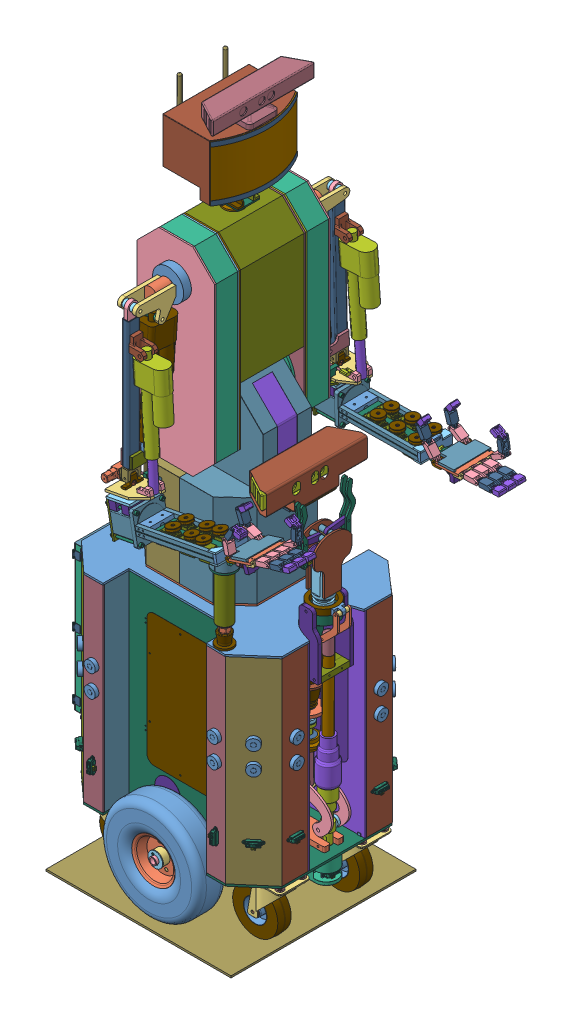
SolidWorks assembly sorbot, configuration По умолчанию. Lengths in mm. (continued)
Components (placement in the parent): (continued)
- bolt1-1: bolt1 [По умолчанию] at (252.2608 28.1179 -56.3731) x (0 0 1) z (1 0 0) size (14 40.5 16.17)
- bolt1-2: bolt1 [По умолчанию] at (172.9115 28.0264 3.3236) x (0 0 1) z (1 0 0) size (14 40.5 16.17)
- bolt1-3: bolt1 [По умолчанию] at (251.9125 28.1164 3.3175) x (0 0 1) z (1 0 0) size (14 40.5 16.17)
- bolt1-4: bolt1 [По умолчанию] at (172.9018 28.0211 -56.2899) x (0 0 1) z (1 0 0) size (14 40.5 16.17)
- bolt1-5: bolt1 [По умолчанию] at (172.7717 28.5111 -218.0055) x (0.546944 0 -0.837169) z (-0.837169 0 -0.546944) size (14 40.5 16.17)
- bolt1-6: bolt1 [По умолчанию] at (251.718 28.5111 -277.7613) x (0.546944 0 -0.837169) z (-0.837169 0 -0.546944) size (14 40.5 16.17)
- bolt1-7: bolt1 [По умолчанию] at (172.7558 28.5111 -277.7529) x (0.546944 0 -0.837169) z (-0.837169 0 -0.546944) size (14 40.5 16.17)
- bolt1-8: bolt1 [По умолчанию] at (251.8056 28.5111 -218.1439) x (0.546944 0 -0.837169) z (-0.837169 0 -0.546944) size (14 40.5 16.17)
- bolt1-9: bolt1 [По умолчанию] at (-260.5376 28.2059 -219.1987) x (0.546944 0 -0.837169) z (-0.837169 0 -0.546944) size (14 40.5 16.17)
- bolt1-10: bolt1 [По умолчанию] at (-181.6432 28.2059 -219.1307) x (0.546944 0 -0.837169) z (-0.837169 0 -0.546944) size (14 40.5 16.17)
- bolt1-11: bolt1 [По умолчанию] at (-181.4767 28.2059 -278.9161) x (0.546944 0 -0.837169) z (-0.837169 0 -0.546944) size (14 40.5 16.17)
- bolt1-12: bolt1 [По умолчанию] at (-260.5141 28.2059 -278.9485) x (0.546944 0 -0.837169) z (-0.837169 0 -0.546944) size (14 40.5 16.17)
- bolt1-13: bolt1 [По умолчанию] at (-260.8842 28.1192 -54.1025) x (-0.546944 0 0.837169) z (0.837169 0 0.546944) size (14 40.5 16.17)
- bolt1-14: bolt1 [По умолчанию] at (-181.8952 28.1192 -54.0898) x (-0.546944 0 0.837169) z (0.837169 0 0.546944) size (14 40.5 16.17)
- bolt1-15: bolt1 [По умолчанию] at (-260.8825 28.1192 5.6198) x (-0.546944 0 0.837169) z (0.837169 0 0.546944) size (14 40.5 16.17)
- bolt1-16: bolt1 [По умолчанию] at (-181.994 28.1192 5.6123) x (-0.546944 0 0.837169) z (0.837169 0 0.546944) size (14 40.5 16.17)
- bolt1.nut-1: bolt1.nut [По умолчанию] at (-181.4767 51.9368 -278.9161) x (0 0 1) z (-1 0 0) size (14 6 16.17)
- bolt1.nut-2: bolt1.nut [По умолчанию] at (-260.5141 51.9368 -278.9485) x (0 0 1) z (-1 0 0) size (14 6 16.17)
- bolt1.nut-3: bolt1.nut [По умолчанию] at (-260.5376 51.9368 -219.1987) x (0 0 1) z (-1 0 0) size (14 6 16.17)
- bolt1.nut-4: bolt1.nut [По умолчанию] at (-181.6432 51.9368 -219.1307) x (0 0 1) z (-1 0 0) size (14 6 16.17)
- bolt1.nut-5: bolt1.nut [По умолчанию] at (-181.994 51.9368 5.6123) x (0 0 -1) z (1 0 0) size (14 6 16.17)
- bolt1.nut-6: bolt1.nut [По умолчанию] at (-260.8825 51.9368 5.6198) x (0 0 -1) z (1 0 0) size (14 6 16.17)
- bolt1.nut-7: bolt1.nut [По умолчанию] at (-260.8842 51.9368 -54.1025) x (0 0 -1) z (1 0 0) size (14 6 16.17)
- bolt1.nut-8: bolt1.nut [По умолчанию] at (-181.8952 51.9368 -54.0898) x (0 0 -1) z (1 0 0) size (14 6 16.17)
- bolt1.nut-9: bolt1.nut [По умолчанию] at (172.9115 51.9368 3.3236) x (0 0 -1) z (1 0 0) size (14 6 16.17)
- bolt1.nut-10: bolt1.nut [По умолчанию] at (251.9125 51.7388 3.3175) x (0 0 -1) z (1 0 0) size (14 6 16.17)
- bolt1.nut-11: bolt1.nut [По умолчанию] at (252.2608 51.5573 -56.3731) x (0 0 -1) z (1 0 0) size (14 6 16.17)
- bolt1.nut-12: bolt1.nut [По умолчанию] at (172.9018 51.3675 -56.2899) x (0 0 -1) z (1 0 0) size (14 6 16.17)
- bolt1.nut-13: bolt1.nut [По умолчанию] at (172.7558 51.9368 -277.7529) x (0 0 1) z (-1 0 0) size (14 6 16.17)
- bolt1.nut-14: bolt1.nut [По умолчанию] at (172.7717 51.9368 -218.0055) x (0 0 1) z (-1 0 0) size (14 6 16.17)
- bolt1.nut-15: bolt1.nut [По умолчанию] at (251.718 51.9368 -277.7613) x (0 0 1) z (-1 0 0) size (14 6 16.17)
- bolt1.nut-16: bolt1.nut [По умолчанию] at (251.8056 51.9368 -218.1439) x (0 0 1) z (-1 0 0) size (14 6 16.17)
- turret.table-1: turret.table [По умолчанию] at (-20.8718 607.7934 -141.039) size (305 5 278)
- turret.center-1: turret.center [По умолчанию] at (-20.0648 607.7934 -136.9555) x (1 0 -0.000338) z (0.000338 0 1) size (90 80 90)
- body.center-1: body.center [По умолчанию] at (-20.0648 627.0246 -136.9555) size (22 355 22)
- wheel.axis.frame.fixture.p1-1: wheel.axis.frame.fixture.p1 [По умолчанию] at (40.6964 23.6368 -47.3934) x (0.999999 0 0.001149) z (-0.001149 0 0.999999) size (21.7 48.8 22.74)
- wheel.axis.frame.fixture.p1-2: wheel.axis.frame.fixture.p1 [По умолчанию] at (-54.5345 23.6368 -47.3503) size (21.7 48.8 22.74)
- wheel.axis.frame.fixture.p1-3: wheel.axis.frame.fixture.p1 [По умолчанию] at (40.6515 23.6368 -224.9519) size (21.7 48.8 22.74)
- wheel.axis.frame.fixture.p1-4: wheel.axis.frame.fixture.p1 [По умолчанию] at (-54.2945 23.6368 -224.8346) size (21.7 48.8 22.74)
- gearmotor.fixture.p2.1-1: gearmotor.fixture.p2.1 [По умолчанию] at (2.1309 53.4368 -208.1692) x (-1 0 0) z (0 0 -1) size (86 101.43 182)
- wheel.axis.frame.fixture.p2-1: wheel.axis.frame.fixture.p2 [По умолчанию] at (40.6964 51.9368 -47.3934) size (22.08 10 22.5)
- wheel.axis.frame.fixture.p2-2: wheel.axis.frame.fixture.p2 [По умолчанию] at (40.6515 53.4933 -224.9519) size (22.08 10 22.5)
- wheel.axis.frame.fixture.p2-3: wheel.axis.frame.fixture.p2 [По умолчанию] at (-54.2945 53.4933 -224.8346) size (22.08 10 22.5)
- wheel.axis.frame.fixture.p2-4: wheel.axis.frame.fixture.p2 [По умолчанию] at (-54.5345 53.4933 -47.3503) size (22.08 10 22.5)
- wall-fixture-3-2: wall-fixture-3 [По умолчанию] at (-150.6756 56.9368 4.4522) size (287.58 65 40)
- wall-fixture-3-1-1: wall-fixture-3-1 [По умолчанию] at (-154.6756 56.9368 4.4522) x (0 0 -1) z (1 0 0) size (74 65 40)
- wall-fixture-3-2-1: wall-fixture-3-2 [По умолчанию] at (-154.6756 56.9368 74.4522) size (42 65 40)
- wall-fixture-3-3-1: wall-fixture-3-3 [По умолчанию] at (-194.4824 56.9368 75.4251) x (0.73854 0 0.67421) z (-0.67421 0 0.73854) size (116.95 65 40)
- ground-1: ground [По умолчанию] at (-17.2598 -128.0632 -134.3184) size (500 5 500)
- body_pivot_fixture-1: body_pivot_fixture [По умолчанию] at (-20.0648 922.0246 -136.9555) x (0.99898 0 -0.04516) z (0.04516 0 0.99898) size (78 60 78)
- body_axis-1: body_axis [По умолчанию] at (-20.0648 1016.5246 -221.0975) x (0.999995 0.003042 0) z (0 0 1) size (21.8 21.8 170.35)
- body.frame.p1.fixture-1: body.frame.p1.fixture [По умолчанию] at (-20.8083 1016.2071 -56.7442) x (-0.989237 -0.146324 0) z (0 0 -1) size (89 89 22)
- body.frame.p1.fixture-2: body.frame.p1.fixture [По умолчанию] at (-20.0648 1016.5246 -216.3595) x (0.862438 0.506162 0) z (0 0 1) size (89 89 22)
- body.frame.p2-1: body.frame.p2 [По умолчанию] at (-4.2156 797.7971 -50.7442) x (-1 0 0) z (0 0 -1) size (210 323.57 171.62)
- body.frame.p3-1: body.frame.p3 [По умолчанию] at (94.3623 1112.7235 -40.8506) x (-1 0 0) z (0 0 -1) size (206 2 171.62)
- arm.actuator-1: arm.actuator [Default] at (-100.027 1094.2768 -11.7544) x (0 0 -1) z (0.997693 -0.067885 0) size (42 292 82)
  - arm.actuator.p1-1: arm.actuator.p1 [Default] at (1.9897 -28.1276 18.0595) size (42 292 82)
- arm.actuator.p2-1: arm.actuator.p2 [Default] at (-71.299 1250.4551 -13.7442) x (-0.997693 0.067885 0) z (0 0 -1) size (20 180 20)
- arm.lift.actuator.fixture.p2-1: arm.lift.actuator.fixture.p2 [По умолчанию] at (-88.5767 993.1387 -41.8307) x (0.99962 0.027553 0) z (0 0 1) size (8 8 57)
- shoulder.p4-1: shoulder.p4 [По умолчанию] at (-12.6529 1335.4871 -25.7442) x (0.590367 -0.807135 0) z (0 0 1) size (124.11 60 4)
- shoulder.p4-2: shoulder.p4 [По умолчанию] at (-12.6483 1335.4904 -1.7442) x (0.590423 -0.807094 0) z (0 0 1) size (124.11 60 4)
- arm.lift.actuator.fixture.p3-1: arm.lift.actuator.fixture.p3 [По умолчанию] at (-88.5767 993.1387 15.2558) x (-1 -0.000227 0) z (0 0 -1) size (39.1 39.1 19)
- arm.lift.actuator.fixture.p3-2: arm.lift.actuator.fixture.p3 [По умолчанию] at (-88.5767 993.1387 -42.7442) x (1 -0.000113 0) z (0 0 1) size (39.1 39.1 19)
- shoulder.p6-1: shoulder.p6 [По умолчанию] at (-12.6457 1335.4135 -42.7442) x (-0.13701 -0.99057 0) z (0 0 1) size (53.6 53.6 22)
- shoulder.p6-2: shoulder.p6 [По умолчанию] at (-12.6483 1335.4904 16.6679) x (-0.526603 0.850111 0) z (0 0 -1) size (53.6 53.6 22)
- body.frame.p5-1: body.frame.p5 [По умолчанию] at (-12.763 795.3888 -42.7442) x (1 0 0) z (0 0 1) size (210 537.69 58)
- arm.actuator-2: arm.actuator [Default] at (-14.7745 1188.0283 105.1323) x (1 0 0) z (0 -0.068351 -0.997661) size (42 292 82)
  - arm.actuator.p1-1: arm.actuator.p1 [Default] at (1.9897 -28.1276 18.0595) size (42 292 82)
- arm.actuator.p2-2: arm.actuator.p2 [Default] at (-12.7848 1126.9341 91.2161) x (0 -0.068351 -0.997661) z (-1 0 0) size (20 180 20)
- arm.actuator100mm..p1-1: arm.actuator100mm..p1 [Default] at (34.2144 1176.4747 140.2746) x (0 0 1) z (0.998134 0.061067 0) size (42 244 82)
- arm.actuator100mm.p2-1: arm.actuator100mm.p2 [Default] at (41.3177 1060.3732 140.2746) x (0.998134 0.061067 0) z (0 0 -1) size (20 130 20)
- body.frame.p1-3: body.frame.p1 [По умолчанию] at (-12.5732 795.4676 -50.7442) x (1 0 0) z (0 0 1) size (210 537.56 4)
- cap-hinge-1: cap-hinge [По умолчанию] at (95.4017 1285.4557 -46.5922) x (0 0 1) z (0 1 0) size (35.83 6 40) (hidden)
- cap-hinge-p1-1: cap-hinge-p1 [По умолчанию] at (95.4017 1326.2182 -46.5922) x (0 0 -1) z (0 -1 0) size (35.83 6 40) (hidden)
- cap-hinge-2: cap-hinge [По умолчанию] at (95.4017 1183.4534 -46.8053) x (0 0 -1) z (0 -1 0) size (35.83 6 40) (hidden)
- cap-hinge-p1-2: cap-hinge-p1 [По умолчанию] at (95.4017 1142.6154 -46.8053) x (0 0 1) z (0 1 0) size (35.83 6 40) (hidden)
- arm.p1.m-1: arm.p1.m [По умолчанию] at (-12.763 1309.7884 140.1602) x (1 0 0) z (0 0 -1) size (18 345 32.5)
- actuator.100.fixture-1: actuator.100.fixture [По умолчанию] at (23.3566 1237.5198 140.1602) x (0 0 1) z (-1 0 0) size (40 40 44)
- forearm.rotate.p9-1: forearm.rotate.p9 [По умолчанию] at (-4.2763 976.7014 103.5825) x (-1 0 0) z (0 0 1) size (18 63 34)
- forearm.rotate.p12-1: forearm.rotate.p12 [По умолчанию] at (-21.7679 963.9 61.4944) x (1 0 0) z (0 0 -1) size (7 35 61.58)
- lower.arm.p2-1: lower.arm.p2 [По умолчанию] at (41.5663 863.9612 178.2746) x (0.982605 0.185706 0) z (0 0 1) size (214 10 10)
- lower.arm.p2-2: lower.arm.p2 [По умолчанию] at (43.7948 852.17 178.2746) x (0.982605 0.185706 0) z (0 0 -1) size (214 10 10)
- lower.arm.p2-3: lower.arm.p2 [По умолчанию] at (41.5663 863.9612 102.2746) x (0.982605 0.185706 0) z (0 0 1) size (214 10 10)
- lower.arm.p2-4: lower.arm.p2 [По умолчанию] at (43.7948 852.17 102.2746) x (0.982605 0.185706 0) z (0 0 -1) size (214 10 10)
- lower.arm.p3-1: lower.arm.p3 [По умолчанию] at (41.8837 856.8973 100.2593) x (0.982605 0.185706 0) z (0 0 1) size (214 2 86)
- HS-311 Hitec Standard Servo and Horn-1: HS-311 Hitec Standard Servo and Horn [Default] at (126.5902 849.0921 157.9974) x (0 0 1) z (-0.982605 -0.185706 0) size (27.94 44.98 53.29)
  - HS-311 Hitec Standard Servo-1: HS-311 Hitec Standard Servo [Default] at origin size (20.32 41.27 53.29)
  - HS-311-p2-1: HS-311-p2 [По умолчанию] at (0 42.485 0) x (0.967717 0 0.252038) z (-0.252038 0 0.967717) size (22.63 6.25 24)
- HS-311 Hitec Standard Servo and Horn-2: HS-311 Hitec Standard Servo and Horn [Default] at (180.6335 859.3059 119.9974) x (0 0 1) z (-0.982605 -0.185706 0) size (27.94 44.98 53.29)
  - HS-311 Hitec Standard Servo-1: HS-311 Hitec Standard Servo [Default] at origin size (20.32 41.27 53.29)
  - HS-311-p2-1: HS-311-p2 [По умолчанию] at (0 42.485 0) x (0.967717 0 0.252038) z (-0.252038 0 0.967717) size (22.63 6.25 24)
- HS-311 Hitec Standard Servo and Horn-3: HS-311 Hitec Standard Servo and Horn [Default] at (126.5902 849.0921 122.4974) x (0 0 1) z (-0.982605 -0.185706 0) size (27.94 44.98 53.29)
  - HS-311 Hitec Standard Servo-1: HS-311 Hitec Standard Servo [Default] at origin size (20.32 41.27 53.29)
  - HS-311-p2-1: HS-311-p2 [По умолчанию] at (0 42.485 0) x (0.967717 0 0.252038) z (-0.252038 0 0.967717) size (22.63 6.25 24)
- HS-311 Hitec Standard Servo and Horn-4: HS-311 Hitec Standard Servo and Horn [Default] at (214.3565 865.6794 117.4346) x (0 0 -1) z (0.982605 0.185706 0) size (27.94 44.98 53.29)
  - HS-311 Hitec Standard Servo-1: HS-311 Hitec Standard Servo [Default] at origin size (20.32 41.27 53.29)
  - HS-311-p2-1: HS-311-p2 [По умолчанию] at (0 42.485 0) x (0.967717 0 0.252038) z (-0.252038 0 0.967717) size (22.63 6.25 24)
- HS-311 Hitec Standard Servo and Horn-5: HS-311 Hitec Standard Servo and Horn [Default] at (180.6335 859.3059 160.9974) x (0 0 1) z (-0.982605 -0.185706 0) size (27.94 44.98 53.29)
  - HS-311 Hitec Standard Servo-1: HS-311 Hitec Standard Servo [Default] at origin size (20.32 41.27 53.29)
  - HS-311-p2-1: HS-311-p2 [По умолчанию] at (0 42.485 0) x (0.967717 0 0.252038) z (-0.252038 0 0.967717) size (22.63 6.25 24)
- HS-311 Hitec Standard Servo and Horn-6: HS-311 Hitec Standard Servo and Horn [Default] at (214.3565 865.6794 163.1146) x (0 0 -1) z (0.982605 0.185706 0) size (27.94 44.98 53.29)
  - HS-311 Hitec Standard Servo-1: HS-311 Hitec Standard Servo [Default] at origin size (20.32 41.27 53.29)
  - HS-311-p2-1: HS-311-p2 [По умолчанию] at (0 42.485 0) x (0.967717 0 0.252038) z (-0.252038 0 0.967717) size (22.63 6.25 24)
- lower.arm.p9-1: lower.arm.p9 [По умолчанию] at (119.1648 888.3816 157.9974) x (0.982605 0.185706 0) z (0 0 1) size (32.15 8 32.15)
- lower.arm.p9-2: lower.arm.p9 [По умолчанию] at (119.1648 888.3816 122.4974) x (0.982605 0.185706 0) z (0 0 1) size (32.15 8 32.15)
- lower.arm.p9-3: lower.arm.p9 [По умолчанию] at (206.9311 904.9689 163.1146) x (-0.982605 -0.185706 0) z (0 0 -1) size (32.15 8 32.15)
- lower.arm.p9-4: lower.arm.p9 [По умолчанию] at (173.2081 898.5954 160.9974) x (0.982605 0.185706 0) z (0 0 1) size (32.15 8 32.15)
- lower.arm.p9-5: lower.arm.p9 [По умолчанию] at (173.2081 898.5954 119.9974) x (0.982605 0.185706 0) z (0 0 1) size (32.15 8 32.15)
- lower.arm.p9-6: lower.arm.p9 [По умолчанию] at (206.9311 904.9689 117.4346) x (-0.982605 -0.185706 0) z (0 0 -1) size (32.15 8 32.15)
- lower.arm.p8-2: lower.arm.p8 [По умолчанию] at (250.9153 908.6154 183.2746) x (0.982605 0.185706 0) z (0 0 1) size (8 36.31 86)
- palm.p1-3: palm.p1 [По умолчанию] at (326.2301 928.273 153.074) x (0.950144 0.311545 0.012888) z (-0.012247 -0.004016 0.999917) size (75 6 100)
- palm.p3-1: palm.p3 [По умолчанию] at (374.5143 939.8955 115.7089) x (-0.012247 -0.004016 0.999917) z (-0.950144 -0.311545 -0.012888) size (100 13.5 26)
- finger.p1-1: finger.p1 [По умолчанию] at (361.4218 946.6526 179.831) x (0.950144 0.311545 0.012888) z (-0.012247 -0.004016 0.999917) size (50 12 20.5)
- palm.fixture.p4-1: palm.fixture.p4 [По умолчанию] at (258.7762 910.1011 183.2746) x (0 0 -1) z (0.982605 0.185706 0) size (25 4 20)
- palm.fixture.p4-3: palm.fixture.p4 [По умолчанию] at (263.6045 884.5534 183.2746) x (0 0 -1) z (0.982605 0.185706 0) size (25 4 20)
- palm.fixture.p4-4: palm.fixture.p4 [По умолчанию] at (258.7762 910.1011 97.2746) x (-0.982605 -0.185706 0) z (0 0 -1) size (25 4 20)
- palm.fixture.p4-5: palm.fixture.p4 [По умолчанию] at (262.8617 888.4838 97.2746) x (0 0 1) z (0.982605 0.185706 0) size (25 4 20)
- finger.spring-1: finger.spring [По умолчанию] at (366.5011 947.2657 178.5056) x (0.311571 -0.950223 0) z (-0.012247 -0.004016 0.999917) size (5.38 21 4.23)
- palm.fixture.p13-1: palm.fixture.p13 [По умолчанию] at (366.3409 947.2132 191.5879) x (0.430913 -0.902392 0.001654) z (0.012247 0.004016 -0.999917) size (3 3 100)
- finger.spring-2: finger.spring [По умолчанию] at (405.9116 957.8496 176.7806) x (0.327007 -0.945022 0.00021) z (-0.012247 -0.004016 0.999917) size (5.38 21 4.23)
- finger.p3-1: finger.p3 [По умолчанию] at (437.7359 970.6062 180.9748) x (0.950144 0.311546 0.012888) z (-0.012247 -0.004016 0.999917) size (30 12 20.5)
- finger.p1-2: finger.p1 [По умолчанию] at (362.6718 945.7123 103.3362) x (0.841955 0.539404 0.012478) z (-0.012247 -0.004016 0.999917) size (50 12 20.5)
- finger.p3-2: finger.p3 [По умолчанию] at (404.7341 1004.7181 104.2012) x (-0.905154 0.424979 -0.00938) z (-0.012247 -0.004016 0.999917) size (30 12 20.5)
- finger.p1-3: finger.p1 [По умолчанию] at (361.7341 946.755 154.3331) x (0.950144 0.311545 0.012888) z (-0.012247 -0.004016 0.999917) size (50 12 20.5)
- finger.p3-3: finger.p3 [По умолчанию] at (437.7976 971.5136 155.4898) x (0.950144 0.311546 0.012888) z (-0.012247 -0.004016 0.999917) size (30 12 20.5)
- palm.p3.m-1: palm.p3.m [По умолчанию] at (294.6906 913.722 190.6324) x (0.012247 0.004016 -0.999917) z (0.950144 0.311545 0.012888) size (21.5 12 26)
- finger.p1-4: finger.p1 [По умолчанию] at (362.0464 946.8574 128.8352) x (0.950144 0.311545 0.012888) z (-0.012247 -0.004016 0.999917) size (50 12 20.5)
- finger.p3-4: finger.p3 [По умолчанию] at (438.0521 971.8022 129.7881) x (0.950144 0.311546 0.012888) z (-0.012247 -0.004016 0.999917) size (30 12 20.5)
- palm.p3.m-2: palm.p3.m [По умолчанию] at (295.652 914.0372 112.1389) x (0.012247 0.004016 -0.999917) z (0.950144 0.311545 0.012888) size (21.5 12 26)
- finger.p1-5: finger.p1 [По умолчанию] at (298.6941 917.8741 179.9472) x (-0.206644 0.978415 0.001398) z (0.012247 0.004016 -0.999917) size (50 12 20.5)
- finger.p3-5: finger.p3 [По умолчанию] at (303.3786 994.7192 180.4261) x (0.98461 -0.174397 0.011359) z (0.012247 0.004016 -0.999917) size (30 12 20.5)
- finger.p1-6: finger.p1 [По умолчанию] at (302.6817 922.0965 101.6065) x (-0.939132 0.343406 -0.010123) z (0.012247 0.004016 -0.999917) size (50 12 20.5)
- finger.p3-6: finger.p3 [По умолчанию] at (242.2623 968.6455 101.1663) x (0.802448 0.596597 0.012224) z (0.012247 0.004016 -0.999917) size (30 12 20.5)
- finger.p2-7: finger.p2 [По умолчанию] at (400.3799 959.5495 180.36) x (0.957938 0.286686 0.012884) z (-0.012247 -0.004016 0.999917) size (48 12 20.5)
- finger.p2-8: finger.p2 [По умолчанию] at (400.6902 959.5494 154.8616) x (0.951517 0.307327 0.012888) z (-0.012247 -0.004016 0.999917) size (48 12 20.5)
- finger.p2-9: finger.p2 [По умолчанию] at (401.0023 959.6281 129.3637) x (0.949969 0.312079 0.012888) z (-0.012247 -0.004016 0.999917) size (48 12 20.5)
- finger.p2-10: finger.p2 [По умолчанию] at (400.3467 964.4738 103.873) x (-0.01257 0.999914 0.003862) z (-0.012247 -0.004016 0.999917) size (48 12 20.5)
- finger.p2-11: finger.p2 [По умолчанию] at (286.7699 957.4574 179.9601) x (0.519178 0.85461 0.009791) z (0.012247 0.004016 -0.999917) size (48 12 20.5)
- finger.p2-12: finger.p2 [По умолчанию] at (262.4973 932.6893 101.1569) x (-0.370677 0.928761 -0.00081) z (0.012247 0.004016 -0.999917) size (48 12 20.5)
- finger1.rod-1: finger1.rod [По умолчанию] at (453.9909 979.577 179.5221) x (0.950144 0.311546 0.012888) z (-0.012247 -0.004016 0.999917) size (196.04 3.19 32.22)
- palm.p5-1: palm.p5 [По умолчанию] at (330.6828 936.0474 170.4076) x (0.950144 0.311545 0.012888) z (-0.012247 -0.004016 0.999917) size (21.8 4 21.8)
- palm.p6-1: palm.p6 [По умолчанию] at (301.0674 926.3367 156.6492) x (0.950144 0.311545 0.012888) z (-0.012247 -0.004016 0.999917) size (13.8 4 13.8)
- palm.p5-2: palm.p5 [По умолчанию] at (331.3758 936.2746 112.4456) x (0.950144 0.311545 0.012888) z (-0.012247 -0.004016 0.999917) size (21.8 4 21.8)
- palm.p6-2: palm.p6 [По умолчанию] at (301.386 926.4412 124.555) x (0.950144 0.311545 0.012888) z (-0.012247 -0.004016 0.999917) size (13.8 4 13.8)
- palm.cap-1: palm.cap [По умолчанию] at (361.9011 946.2836 191.5864) x (0.950144 0.311545 0.012888) z (-0.012247 -0.004016 0.999917) size (62.89 6 100)
- palm.fixture.p14-1: palm.fixture.p14 [По умолчанию] at (275.8203 911.7441 155.3904) x (0.950144 0.311545 0.012888) z (-0.012247 -0.004016 0.999917) size (45 6 30)
- forearm.rotate.p12-m-1: forearm.rotate.p12-m [По умолчанию] at (3.237 963.9 61.4944) x (1 0 0) z (0 0 -1) size (7 30.01 61.58)
- arm.fixture.cap-1: arm.fixture.cap [По умолчанию] at (-12.4559 1335.4922 -51.2442) x (0.999995 -0.003183 0) z (0.003183 0.999995 0) size (110 23 110)
- body_tilit_stud-1: body_tilit_stud [По умолчанию] at (-48.2188 648.7352 -136.446) x (1 0 -0.000338) z (0.000338 0 1) size (6 307 6)
- shoulder.bearing.housing-1: shoulder.bearing.housing [По умолчанию] at (-12.7629 1335.3853 19.2558) x (1 0 0) z (0 0 1) size (84 84 21)
- shoulder.bearing.housing-2: shoulder.bearing.housing [По умолчанию] at (-12.4903 1335.516 -46.7442) x (-0.799769 0.600308 0) z (0 0 -1) size (84 84 21)
- shoulder.axis-1: shoulder.axis [По умолчанию] at (-12.7629 1335.3853 -67.7442) x (1 0 0) z (0 0 1) size (30 40 157)
- arm.fixture-2: arm.fixture [По умолчанию] at (-27.7629 1348.6141 44.2558) x (-1 0 0) z (0 0 -1) size (10 73.07 108.23)
- shoulder.lever-1: shoulder.lever [По умолчанию] at (-7.763 1350.5713 104.4102) x (-1 0 0) z (0 0 -1) size (10 77.8 28.5)
- arm.lift2.actuator.fixture.p1-1: arm.lift2.actuator.fixture.p1 [По умолчанию] at (-27.763 1335.3853 140.1602) x (1 0 0) z (0 -0.000978 1) size (10 20 20)
- arm.lift2.actuator.fixture.p1.m1-1: arm.lift2.actuator.fixture.p1.m1 [По умолчанию] at (-27.7629 1286.6873 80.2712) x (1 0 0) z (0 -0.000962 1) size (5 20 20)
- arm.fixture-3: arm.fixture [По умолчанию] at (12.2371 1348.614 44.2558) x (-1 0 0) z (0 0 -1) size (10 73.07 108.23)
- arm.lift2.actuator.fixture.p1-3: arm.lift2.actuator.fixture.p1 [По умолчанию] at (-7.7629 1335.3853 140.1602) x (1 0 0) z (0 -0.000978 1) size (10 20 20)
- arm.lift2.actuator.fixture.p1.m1-2: arm.lift2.actuator.fixture.p1.m1 [По умолчанию] at (-2.7629 1286.6873 80.2712) x (1 0 0) z (0 -0.000962 1) size (5 20 20)
- body_pivot-2: body_pivot [По умолчанию] at (-55.8885 972.0246 -153.8981) x (1 0 0) z (0 0 1) size (140 10 130)
- body.tilt.axis.frame-2: body.tilt.axis.frame [По умолчанию] at (29.9352 1018.0246 -79.5942) x (-1 0 0) z (0 0 -1) size (126 65.5 38)
- body.tilt.axis.frame-3: body.tilt.axis.frame [По умолчанию] at (-70.0648 1018.0246 -194.4875) x (1 0 0) z (0 0 1) size (126 65.5 38)
- tilt.thread.rod-1: tilt.thread.rod [По умолчанию] at (-119.3768 729.5591 -141.6211) x (0.714335 0 -0.699804) z (0.699804 0 0.714335) size (16 154 16)
- tilt.thread.rod.fixture.2-1: tilt.thread.rod.fixture.2 [По умолчанию] at (-119.3768 793.5591 -141.6211) size (40 26 40)
- tilit.thread.rod.bearing.fixture-1: tilit.thread.rod.bearing.fixture [По умолчанию] at (-130.6447 929.0246 -154.0466) x (0.999985 0 0.005494) z (-0.005494 0 0.999985) size (171.17 8 70)
- tilit.thread.bearing-1: tilit.thread.bearing [По умолчанию] at (-119.3768 937.0246 -141.6211) size (28 8 28)
- tilit.thread.rod.bearing.housing-1: tilit.thread.rod.bearing.housing [По умолчанию] at (-119.3768 937.0246 -141.6211) size (42.5 10 42.5)
- body_tilt_axis_clamp-1: body_tilt_axis_clamp [По умолчанию] at (-20.0648 1016.5246 -90.4875) x (-0.92275 -0.3854 0) z (0 0 -1) size (65 65 23)
- body_tilt_axis_clamp-2: body_tilt_axis_clamp [По умолчанию] at (-20.0648 1016.5246 -183.5942) x (0.999995 0.003042 0) z (0 0 1) size (65 65 23)
- body_tilt_lever-1: body_tilt_lever [По умолчанию] at (-20.0648 1016.5246 -155.4875) x (0.894303 0.447461 0) z (0 0 1) size (137.08 65 6)
- body_tilt_lever-2: body_tilt_lever [По умолчанию] at (-20.0648 1016.5246 -124.5942) x (0.894303 0.447461 0) z (0 0 1) size (137.08 65 6)
- body.tilit.lever.2-1: body.tilit.lever.2 [По умолчанию] at (-119.3768 828.3995 -181.4655) x (0.133707 0.991021 0) z (-0.991021 0.133707 0) size (179.8 7 30)
- body_tilt_lever_axis-1: body_tilt_lever_axis [По умолчанию] at (-99.3474 976.856 -195.4875) x (-0.131453 -0.991322 0) z (0 0 1) size (10 10 115)
- body.tilt.nut-1: body.tilt.nut [По умолчанию] at (-119.3768 828.3995 -141.6211) x (1 0 -0.000625) z (0.000625 0 1) size (36 14 31.19)
- body.tilit.nut.housing-1: body.tilit.nut.housing [По умолчанию] at (-119.3768 818.3995 -141.6211) x (0 0 -1) z (1 0 0) size (79.69 20 43.97)
- body.tilit.nut.housing.bolt-1: body.tilit.nut.housing.bolt [По умолчанию] at (-119.3768 828.3995 -188.4655) x (0 0 1) z (-1 0 0) size (38 19.4 20.53)
- body.tilit.nut.housing.cap-1: body.tilit.nut.housing.cap [По умолчанию] at (-97.3898 838.3995 -181.4655) x (0 0 1) z (-1 0 0) size (79.69 10 43.97)
- body.tilit.extender-1: body.tilit.extender [По умолчанию] at (-99.3474 976.856 -155.4875) x (0 0 -1) z (1 0 0) size (21.5 30 30)
- washer-1: washer [По умолчанию] at (-99.3474 976.856 -190.4655) x (1 0 0) z (0 0 1) size (24 24 2)
- body.tilit.extender-2: body.tilit.extender [По умолчанию] at (-99.3474 976.856 -97.0942) x (0 0 -1) z (1 0 0) size (21.5 30 30)
- body.tilit.lever.2-2: body.tilit.lever.2 [По умолчанию] at (-119.3768 828.3995 -94.7768) x (0.133707 0.991021 0) z (-0.991021 0.133707 0) size (179.8 7 30)
- body.tilit.nut.housing.bolt-2: body.tilit.nut.housing.bolt [По умолчанию] at (-119.3768 828.3995 -94.7768) x (0 0 -1) z (1 0 0) size (38 19.4 20.53)
- washer-2: washer [По умолчанию] at (-99.3474 976.856 -94.7768) x (1 0 0) z (0 0 1) size (24 24 2)
- body.tilit.enforcement-1: body.tilit.enforcement [По умолчанию] at (-20.8083 1016.2071 -56.7442) x (0.999986 -0.005204 0) z (-0.005204 -0.999986 0) size (178 6 178)
- body.tilit.enforcement-2: body.tilit.enforcement [По умолчанию] at (-20.0648 1016.5246 -222.3595) x (1 0 0) z (0 -1 0) size (178 6 178)
- arm.fixture.cap-2: arm.fixture.cap [По умолчанию] at (-15.2428 1335.4923 -221.8595) x (0.999986 -0.005204 0) z (-0.005204 -0.999986 0) size (110 23 110)
- body.frame.p4-4: body.frame.p4 [По умолчанию] at (-12.3773 795.5195 -230.3595) x (1 0 0) z (0 0 1) size (210 537.56 4)
- body.frame.p5-2: body.frame.p5 [По умолчанию] at (-12.6499 795.3889 -288.3595) x (1 0 0) z (0 0 1) size (210 537.69 58)
- cap-hinge-p1-3: cap-hinge-p1 [По умолчанию] at (95.5097 1287.1115 -226.3787) x (0 0 1) z (0 1 0) size (35.83 6 40) (hidden)
- cap-hinge-4: cap-hinge [По умолчанию] at (95.5097 1143.1735 -226.3787) x (0 0 1) z (0 1 0) size (35.83 6 40) (hidden)
- cap-hinge-5: cap-hinge [По умолчанию] at (95.5097 1327.9494 -226.3787) x (-0.005204 0 -0.999986) z (0 -1 0) size (35.83 6 40) (hidden)
- cap-hinge-p1-4: cap-hinge-p1 [По умолчанию] at (95.5097 1183.936 -226.3787) x (-0.005211 0 -0.999986) z (0 -1 0) size (35.83 6 40) (hidden)
- shoulder.bearing.housing-3: shoulder.bearing.housing [По умолчанию] at (-12.6499 1335.3853 -292.3595) x (1 -0.000001 0) z (0 0 -1) size (84 84 21)
- shoulder.bearing.housing-4: shoulder.bearing.housing [По умолчанию] at (-12.3772 1335.516 -226.3595) x (1 0 0) z (0 0 1) size (84 84 21)
- shoulder.axis-2: shoulder.axis [По умолчанию] at (-12.6499 1335.3853 -205.3595) x (1 0 0) z (0 0 -1) size (30 40 157)
- shoulder.p6-3: shoulder.p6 [По умолчанию] at (-12.6499 1335.3853 -227.2739) x (-0.950595 -0.310432 0) z (0 0 -1) size (53.6 53.6 22)
- shoulder.p6-4: shoulder.p6 [По умолчанию] at (-12.6499 1335.3853 -288.3595) x (1 0 0) z (0 0 1) size (53.6 53.6 22)
- shoulder.p4-3: shoulder.p4 [По умолчанию] at (-12.6499 1335.3853 -247.3595) x (0.588806 -0.808274 0) z (0 0 1) size (124.11 60 4)
- shoulder.p4-4: shoulder.p4 [По умолчанию] at (-12.6499 1335.3853 -268.3595) x (0.588806 -0.808274 0) z (0 0 1) size (124.11 60 4)
- arm.lift.actuator.fixture.p3-3: arm.lift.actuator.fixture.p3 [По умолчанию] at (-88.5702 993.1387 -230.3595) x (-0.619572 -0.78494 0) z (0 0 -1) size (39.1 39.1 19)
- arm.lift.actuator.fixture.p3-4: arm.lift.actuator.fixture.p3 [По умолчанию] at (-88.5702 993.1387 -288.3595) x (0.977487 0.210996 0) z (0 0 1) size (39.1 39.1 19)
- arm.lift.actuator.fixture.p2-2: arm.lift.actuator.fixture.p2 [По умолчанию] at (-88.5702 993.1387 -287.3595) x (0.873274 0.487229 0) z (0 0 1) size (8 8 57)
- arm.actuator-4: arm.actuator [Default] at (-99.8169 1094.2584 -257.3698) x (0 0 -1) z (0.997711 -0.067628 0) size (42 292 82)
  - arm.actuator.p1-1: arm.actuator.p1 [Default] at (1.9897 -28.1276 18.0595) size (42 292 82)
- arm.actuator.p2-4: arm.actuator.p2 [Default] at (-71.1292 1250.4441 -259.3595) x (0.997711 -0.067628 0) z (0 0 1) size (20 180 20)
- arm.fixture-4: arm.fixture [По умолчанию] at (2.3501 1348.6141 -317.3595) x (0.999986 0 0.005196) z (-0.005196 -0.000016 0.999986) size (10 73.07 108.23)
- arm.fixture-5: arm.fixture [По умолчанию] at (-37.6497 1348.6141 -317.4115) x (0.999986 0 0.005196) z (-0.005196 -0.000016 0.999986) size (10 73.07 108.23)
- shoulder.lever-2: shoulder.lever [По умолчанию] at (-17.3387 1349.7788 -377.2903) x (0.999986 0 0.005196) z (-0.005195 -0.022106 0.999742) size (10 77.8 28.5)
- arm.lift2.actuator.fixture.p1-4: arm.lift2.actuator.fixture.p1 [По умолчанию] at (-7.1514 1335.3868 -413.3148) x (0.999986 0 0.005196) z (-0.005196 -0.000016 0.999986) size (10 20 20)
- arm.lift2.actuator.fixture.p1-5: arm.lift2.actuator.fixture.p1 [По умолчанию] at (-27.1515 1335.3868 -413.2628) x (0.999986 0 0.005196) z (-0.005196 0 0.999986) size (10 20 20)
- arm.p1.m-2: arm.p1.m [По умолчанию] at (-12.1088 964.8834 -421.5332) x (0.999986 0 0.005196) z (-0.005195 -0.022106 0.999742) size (18 345 32.5)
- arm.actuator-5: arm.actuator [Default] at (-10.3307 1188.6881 -380.7869) x (-0.999986 0 -0.005196) z (-0.005174 -0.093519 0.995604) size (42 292 82)
  - arm.actuator.p1-1: arm.actuator.p1 [Default] at (1.9897 -28.1276 18.0595) size (42 292 82)
- arm.lift2.actuator.fixture.p1.m1-3: arm.lift2.actuator.fixture.p1.m1 [По умолчанию] at (-2.4627 1286.6879 -353.4014) x (0.999986 0 0.005196) z (-0.005196 0 0.999986) size (5 20 20)
- arm.lift2.actuator.fixture.p1.m1-4: arm.lift2.actuator.fixture.p1.m1 [По умолчанию] at (-27.4627 1286.6879 -353.3754) x (0.999986 0 0.005196) z (-0.005196 0 0.999986) size (5 20 20)
- forearm.rotate.p12-m-2: forearm.rotate.p12-m [По умолчанию] at (-28.517 962.2566 -343.0069) x (-0.999986 0 -0.005196) z (-0.005195 -0.022106 0.999742) size (7 30.01 61.58)
- forearm.rotate.p12-2: forearm.rotate.p12 [По умолчанию] at (-3.5174 962.2566 -342.877) x (-0.999986 0 -0.005196) z (-0.005195 -0.022106 0.999742) size (7 35 61.58)
- forearm.rotate.p9-2: forearm.rotate.p9 [По умолчанию] at (-3.6751 977.684 -457.5619) x (-0.999986 0 -0.005196) z (-0.005195 -0.022106 0.999742) size (18 63 34)
- actuator.100.fixture-2: actuator.100.fixture [По умолчанию] at (23.979 1237.6167 -415.315) x (-0.005195 -0.022106 0.999742) z (-0.999986 0 -0.005196) size (40 40 44)
- arm.actuator100mm..p1-2: arm.actuator100mm..p1 [Default] at (34.5587 1176.5672 -416.4955) x (-0.005195 -0.022106 0.999742) z (0.998347 0.057103 0.006451) size (42 244 82)
- arm.actuator100mm.p2-2: arm.actuator100mm.p2 [Default] at (41.821 1049.9101 -419.2584) x (0.998347 0.057103 0.006451) z (0.005195 0.022106 -0.999742) size (20 130 20)
- lower.arm.p2-5: lower.arm.p2 [По умолчанию] at (28.9806 854.5589 -385.1362) x (0.99991 0.012267 0.005467) z (-0.005195 -0.022106 0.999742) size (214 10 10)
- lower.arm.p2-6: lower.arm.p2 [По умолчанию] at (29.1292 842.5627 -385.4007) x (0.99991 0.012267 0.005467) z (-0.005195 -0.022106 0.999742) size (214 10 10)
- lower.arm.p2-7: lower.arm.p2 [По умолчанию] at (29.3754 856.2389 -461.1166) x (0.99991 0.012267 0.005467) z (-0.005195 -0.022106 0.999742) size (214 10 10)
- lower.arm.p2-8: lower.arm.p2 [По умолчанию] at (29.524 844.2428 -461.3811) x (0.99991 0.012267 0.005467) z (-0.005195 -0.022106 0.999742) size (214 10 10)
- lower.arm.p3-2: lower.arm.p3 [По умолчанию] at (28.4727 849.2735 -463.2911) x (0.99991 0.012267 0.005467) z (-0.005195 -0.022106 0.999742) size (214 2 86)
- lower.arm.p8-3: lower.arm.p8 [По умолчанию] at (242.8734 862.0719 -378.8573) x (0.99991 0.012267 0.005467) z (-0.005195 -0.022106 0.999742) size (8 36.31 86)
- HS-311 Hitec Standard Servo and Horn-7: HS-311 Hitec Standard Servo and Horn [Default] at (166.093 826.2367 -402.7745) x (-0.005195 -0.022106 0.999742) z (-0.99991 -0.012267 -0.005467) size (27.94 44.98 53.29)
  - HS-311 Hitec Standard Servo-1: HS-311 Hitec Standard Servo [Default] at origin size (20.32 41.27 53.29)
  - HS-311-p2-1: HS-311-p2 [По умолчанию] at (0 42.485 0) x (0.967717 0 0.252038) z (-0.252038 0 0.967717) size (22.63 6.25 24)
- HS-311 Hitec Standard Servo and Horn-8: HS-311 Hitec Standard Servo and Horn [Default] at (166.3037 827.1333 -443.3241) x (-0.005195 -0.022106 0.999742) z (-0.99991 -0.012267 -0.005467) size (27.94 44.98 53.29)
  - HS-311 Hitec Standard Servo-1: HS-311 Hitec Standard Servo [Default] at origin size (20.32 41.27 53.29)
  - HS-311-p2-1: HS-311-p2 [По умолчанию] at (0 42.485 0) x (0.967717 0 0.252038) z (-0.252038 0 0.967717) size (22.63 6.25 24)
- HS-311 Hitec Standard Servo and Horn-9: HS-311 Hitec Standard Servo and Horn [Default] at (221.0839 826.8549 -399.9145) x (-0.005195 -0.022106 0.999742) z (-0.99991 -0.012267 -0.005467) size (27.94 44.98 53.29)
  - HS-311 Hitec Standard Servo-1: HS-311 Hitec Standard Servo [Default] at origin size (20.32 41.27 53.29)
  - HS-311-p2-1: HS-311-p2 [По умолчанию] at (0 42.485 0) x (0.967717 0 0.252038) z (-0.252038 0 0.967717) size (22.63 6.25 24)
- HS-311 Hitec Standard Servo and Horn-10: HS-311 Hitec Standard Servo and Horn [Default] at (221.3213 827.8647 -445.5827) x (-0.005195 -0.022106 0.999742) z (-0.99991 -0.012267 -0.005467) size (27.94 44.98 53.29)
  - HS-311 Hitec Standard Servo-1: HS-311 Hitec Standard Servo [Default] at origin size (20.32 41.27 53.29)
  - HS-311-p2-1: HS-311-p2 [По умолчанию] at (0 42.485 0) x (0.967717 0 0.252038) z (-0.252038 0 0.967717) size (22.63 6.25 24)
- HS-311 Hitec Standard Servo and Horn-11: HS-311 Hitec Standard Servo and Horn [Default] at (111.1025 825.6202 -405.7146) x (-0.005195 -0.022106 0.999742) z (-0.99991 -0.012267 -0.005467) size (27.94 44.98 53.29)
  - HS-311 Hitec Standard Servo-1: HS-311 Hitec Standard Servo [Default] at origin size (20.32 41.27 53.29)
  - HS-311-p2-1: HS-311-p2 [По умолчанию] at (0 42.485 0) x (0.967717 0 0.252038) z (-0.252038 0 0.967717) size (22.63 6.25 24)
- HS-311 Hitec Standard Servo and Horn-12: HS-311 Hitec Standard Servo and Horn [Default] at (111.2858 826.4002 -440.9855) x (-0.005195 -0.022106 0.999742) z (-0.99991 -0.012267 -0.005467) size (27.94 44.98 53.29)
  - HS-311 Hitec Standard Servo-1: HS-311 Hitec Standard Servo [Default] at origin size (20.32 41.27 53.29)
  - HS-311-p2-1: HS-311-p2 [По умолчанию] at (0 42.485 0) x (0.967717 0 0.252038) z (-0.252038 0 0.967717) size (22.63 6.25 24)
- lower.arm.p9-7: lower.arm.p9 [По умолчанию] at (110.6073 865.5925 -404.8333) x (0.99855 0.01352 -0.052116) z (0.052397 -0.021363 0.998398) size (32.15 8 32.15)
- lower.arm.p9-8: lower.arm.p9 [По умолчанию] at (110.7906 866.3724 -440.1042) x (0.99855 0.01352 -0.052116) z (0.052397 -0.021363 0.998398) size (32.15 8 32.15)
- lower.arm.p9-9: lower.arm.p9 [По умолчанию] at (165.5978 866.2089 -401.8932) x (0.99855 0.01352 -0.052116) z (0.052397 -0.021363 0.998398) size (32.15 8 32.15)
- lower.arm.p9-10: lower.arm.p9 [По умолчанию] at (165.8085 867.1056 -442.4428) x (0.99855 0.01352 -0.052116) z (0.052397 -0.021363 0.998398) size (32.15 8 32.15)
- lower.arm.p9-11: lower.arm.p9 [По умолчанию] at (220.5887 866.8271 -399.0332) x (0.99855 0.01352 -0.052116) z (0.052397 -0.021363 0.998398) size (32.15 8 32.15)
- lower.arm.p9-12: lower.arm.p9 [По умолчанию] at (220.826 867.837 -444.7014) x (0.99855 0.01352 -0.052116) z (0.052397 -0.021363 0.998398) size (32.15 8 32.15)
- palm.fixture.p4-6: palm.fixture.p4 [По умолчанию] at (250.8727 862.1701 -378.8136) x (0.005195 0.022106 -0.999742) z (0.99991 0.012267 0.005467) size (25 4 20)
- palm.fixture.p4-7: palm.fixture.p4 [По умолчанию] at (251.1947 836.1784 -379.3866) x (0.005195 0.022106 -0.999742) z (0.99991 0.012267 0.005467) size (25 4 20)
- palm.fixture.p4-8: palm.fixture.p4 [По умолчанию] at (251.2699 868.0699 -464.7032) x (-0.005195 -0.022106 0.999742) z (0.99991 0.012267 0.005467) size (25 4 20)
- palm.fixture.p4-9: palm.fixture.p4 [По умолчанию] at (251.5919 842.0782 -465.2763) x (-0.005195 -0.022106 0.999742) z (0.99991 0.012267 0.005467) size (25 4 20)
- palm.fixture.p14-2: palm.fixture.p14 [По умолчанию] at (269.4564 861.0224 -406.5181) x (0.998179 0.059975 0.006513) z (-0.005195 -0.022106 0.999742) size (45 6 30)
- palm.p1-4: palm.p1 [По умолчанию] at (322.3917 864.2684 -409.1721) x (0.998179 0.059975 0.006513) z (-0.005195 -0.022106 0.999742) size (75 6 100)
- palm.p6-3: palm.p6 [По умолчанию] at (295.9379 868.6488 -407.401) x (0.998026 0.059682 0.019549) z (-0.018211 -0.022887 0.999572) size (13.8 4 13.8)
- palm.p6-4: palm.p6 [По умолчанию] at (296.3955 869.3003 -436.0217) x (0.998026 0.059682 0.019549) z (-0.018211 -0.022887 0.999572) size (13.8 4 13.8)
- palm.p5-3: palm.p5 [По умолчанию] at (330.0768 870.2924 -388.4794) x (0.998026 0.059682 0.019549) z (-0.018211 -0.022887 0.999572) size (21.8 4 21.8)
- palm.p5-4: palm.p5 [По умолчанию] at (330.5285 871.7398 -453.6282) x (0.998026 0.059682 0.019549) z (-0.018211 -0.022887 0.999572) size (21.8 4 21.8)
- palm.cap-2: palm.cap [По умолчанию] at (361.6475 871.8083 -370.7916) x (0.998179 0.059975 0.006513) z (-0.005195 -0.022106 0.999742) size (62.89 6 100)
- palm.p3.m-3: palm.p3.m [По умолчанию] at (288.4804 857.3964 -371.4904) x (0.005195 0.022106 -0.999742) z (0.998179 0.059975 0.006513) size (21.5 12 26)
- palm.p3.m-4: palm.p3.m [По умолчанию] at (288.8882 859.1317 -449.9702) x (0.005195 0.022106 -0.999742) z (0.998179 0.059975 0.006513) size (21.5 12 26)
- palm.p3-2: palm.p3 [По умолчанию] at (371.7565 864.0564 -446.93) x (-0.005195 -0.022106 0.999742) z (-0.998179 -0.059975 -0.006513) size (100 13.5 26)
- finger.p1-7: finger.p1 [По умолчанию] at (296.4475 862.3561 -382.0921) x (-0.618608 0.785572 0.014156) z (0.005195 0.022106 -0.999742) size (50 12 20.5)
- finger.p2-13: finger.p2 [По умолчанию] at (270.5619 893.9062 -381.529) x (-0.470174 0.882409 0.017069) z (0.005195 0.022106 -0.999742) size (48 12 20.5)
- finger.p3-7: finger.p3 [По умолчанию] at (247.3729 927.0618 -381.0293) x (0.5845 0.811122 0.020973) z (0.005195 0.022106 -0.999742) size (30 12 20.5)
- finger.p1-8: finger.p1 [По умолчанию] at (297.7094 865.5037 -460.5362) x (-0.837201 0.54684 0.007741) z (0.005195 0.022106 -0.999742) size (50 12 20.5)
- finger.p2-14: finger.p2 [По умолчанию] at (261.4158 885.1756 -460.2898) x (-0.260238 0.965337 0.019993) z (0.005195 0.022106 -0.999742) size (48 12 20.5)
- finger.p3-8: finger.p3 [По умолчанию] at (247.2354 922.2478 -459.4309) x (0.584142 0.81138 0.020977) z (0.005195 0.022106 -0.999742) size (30 12 20.5)
- finger.p1-9: finger.p1 [По умолчанию] at (361.3008 872.5443 -382.5301) x (0.998179 0.059975 0.006513) z (-0.005195 -0.022106 0.999742) size (50 12 20.5)
- finger.p2-15: finger.p2 [По умолчанию] at (402.2262 875.0033 -382.2631) x (0.998179 0.059975 0.006513) z (-0.005195 -0.022106 0.999742) size (48 12 20.5)
- finger.p3-9: finger.p3 [По умолчанию] at (441.1545 877.3398 -381.8962) x (0.998179 0.059975 0.006513) z (-0.005195 -0.022106 0.999742) size (30 12 20.5)
- finger.p1-10: finger.p1 [По умолчанию] at (361.4333 873.108 -408.0235) x (0.998179 0.059975 0.006513) z (-0.005195 -0.022106 0.999742) size (50 12 20.5)
- finger.p2-16: finger.p2 [По умолчанию] at (402.3586 875.567 -407.7565) x (0.998179 0.059975 0.006513) z (-0.005195 -0.022106 0.999742) size (48 12 20.5)
- finger.p3-10: finger.p3 [По умолчанию] at (441.287 877.9035 -407.3897) x (0.998179 0.059975 0.006513) z (-0.005195 -0.022106 0.999742) size (30 12 20.5)
- finger.p1-11: finger.p1 [По умолчанию] at (361.5658 873.6717 -433.517) x (0.998179 0.059975 0.006513) z (-0.005195 -0.022106 0.999742) size (50 12 20.5)
- finger.p2-17: finger.p2 [По умолчанию] at (402.4911 876.1307 -433.2499) x (0.998179 0.059975 0.006513) z (-0.005195 -0.022106 0.999742) size (48 12 20.5)
- finger.p3-11: finger.p3 [По умолчанию] at (441.4195 878.4672 -432.8831) x (0.998179 0.059975 0.006513) z (-0.005195 -0.022106 0.999742) size (30 12 20.5)
- finger.p1-12: finger.p1 [По умолчанию] at (362.0023 871.6766 -459.0654) x (0.841263 0.540379 0.01632) z (-0.005195 -0.022106 0.999742) size (50 12 20.5)
- finger.p2-18: finger.p2 [По умолчанию] at (400.262 890.3329 -458.454) x (-0.145622 0.989115 0.021115) z (-0.005195 -0.022106 0.999742) size (48 12 20.5)
- finger.p3-12: finger.p3 [По умолчанию] at (398.5933 930.0583 -457.4714) x (-0.870974 0.491289 0.006338) z (-0.005195 -0.022106 0.999742) size (30 12 20.5)
- bodu.tilit.axis.enforcement-1: bodu.tilit.axis.enforcement [По умолчанию] at (-20.0648 1016.5246 -221.0975) x (1 0 0) z (0 0 1) size (18 18 170.35)
- body_tilit_stud-5: body_tilit_stud [По умолчанию] at (-33.7006 648.7352 -112.3187) x (0.499707 0 -0.866195) z (0.866195 0 0.499707) size (6 307 6)
- body_tilit_stud-6: body_tilit_stud [По умолчанию] at (-5.5466 648.7352 -112.8281) x (-0.500293 0 -0.865856) z (0.865856 0 -0.500293) size (6 307 6)
- body_tilit_stud-7: body_tilit_stud [По умолчанию] at (8.0892 648.7352 -137.4649) x (-1 0 0.000338) z (-0.000338 0 -1) size (6 307 6)
- body_tilit_stud-8: body_tilit_stud [По умолчанию] at (-6.429 648.7352 -161.5923) x (-0.499707 0 0.866195) z (-0.866195 0 -0.499707) size (6 307 6)
- body_tilit_stud-9: body_tilit_stud [По умолчанию] at (-34.583 648.7352 -161.0828) x (0.500293 0 0.865856) z (-0.865856 0 0.500293) size (6 307 6)
- m6.nut-1: m6.nut [По умолчанию] at (8.0892 944.0246 -137.4649) size (10 5.5 11.55)
- m6.nut-2: m6.nut [По умолчанию] at (-6.429 944.0246 -161.5923) size (10 5.5 11.55)
- m6.nut-3: m6.nut [По умолчанию] at (-48.2188 944.0246 -136.446) size (10 5.5 11.55)
- m6.nut-4: m6.nut [По умолчанию] at (-34.583 944.0246 -161.0828) size (10 5.5 11.55)
- m6.nut-5: m6.nut [По умолчанию] at (-5.5466 944.0246 -112.8281) size (10 5.5 11.55)
- m6.nut-6: m6.nut [По умолчанию] at (-33.7006 944.0246 -112.3187) size (10 5.5 11.55)
- m6.nut-7: m6.nut [По умолчанию] at (-5.5466 657.2934 -112.8281) size (10 5.5 11.55)
- m6.nut-8: m6.nut [По умолчанию] at (-34.583 657.2934 -161.0828) size (10 5.5 11.55)
- m6.nut-9: m6.nut [По умолчанию] at (8.0892 657.2934 -137.4649) size (10 5.5 11.55)
- m6.nut-10: m6.nut [По умолчанию] at (-6.429 657.2934 -161.5923) size (10 5.5 11.55)
- m6.nut-11: m6.nut [По умолчанию] at (-33.7006 657.2934 -112.3187) size (10 5.5 11.55)
- m6.nut-12: m6.nut [По умолчанию] at (-48.2188 657.2934 -136.446) size (10 5.5 11.55)
- body.tilt.intermediate.enforce-1: body.tilt.intermediate.enforce [По умолчанию] at (-99.3474 976.856 -124.5942) x (1 0 0) z (0 1 0) size (30 25 30)
- arm.drive.p2-1: arm.drive.p2 [По умолчанию] at (43.6014 1241.2974 -35.5806) x (-0.089772 0 -0.995962) z (0.995962 0 -0.089772) size (134 5 24)
- arm.drive.p3-1: arm.drive.p3 [По умолчанию] at (3.7745 1243.7974 -50.7442) x (0 0 -1) z (0.174973 -0.984573 0) size (133.1 20 20)
- body.frame.p1-left-1: body.frame.p1-left [По умолчанию] at (-12.5682 795.4677 -226.3595) x (1 0 0) z (0 0 1) size (210 537.56 4)
- arm.drive.motor-1: arm.drive.motor [По умолчанию] at (-94.8762 1249.003 -67.2442) x (-0.533544 -0.845772 0) z (0.845772 -0.533544 0) size (117 39.5 152)
- arm.drive.motor.pair-1: arm.drive.motor.pair [По умолчанию] at (-76.8976 1162.9951 -205.8595) x (-0.885964 0.463755 0) z (0.463755 0.885964 0) size (117 39.5 152)
- arm.actuator.p2-5: arm.actuator.p2 [Default] at (-12.384 1125.8641 -368.5595) x (-0.005174 -0.093519 0.995604) z (0.999986 0 0.005196) size (20 180 20)
- arm.drive.p5-1: arm.drive.p5 [По умолчанию] at (3.7745 1243.7974 -58.7442) x (1 0 0) z (0 -1 0) size (34 8 34)
- arm.drive.p6-1: arm.drive.p6 [По умолчанию] at (3.7745 1243.7974 -50.7442) x (1 0 0) z (0 1 0) size (40 12 40)
- arm.drive.p3-2: arm.drive.p3 [По умолчанию] at (-20.8275 1162.0905 -222.3595) x (0 0 1) z (-0.923728 -0.383049 0) size (133.1 20 20)
- arm.drive.p5-2: arm.drive.p5 [По умолчанию] at (-20.8275 1162.0905 -214.3595) x (1 0 0) z (0 1 0) size (34 8 34)
- arm.drive.p6-2: arm.drive.p6 [По умолчанию] at (-20.8275 1162.0905 -222.3595) x (1 0.000029 0) z (0.000029 -1 0) size (40 12 40)
- arm.drive.p2-pair-1: arm.drive.p2-pair [По умолчанию] at (50.3811 1159.5904 -236.7848) x (-0.315418 0 0.948953) z (-0.948953 0 -0.315418) size (144 5 24)
- m14.nut-1: m14.nut [По умолчанию] at (-20.8275 1162.0905 -118.4852) x (0.513607 -0.858026 0) z (0.858026 0.513607 0) size (25.4 10.5 22.2)
- arm.drive.p7-2: arm.drive.p7 [По умолчанию] at (-14.5918 1147.0905 -123.4852) x (0 0 1) z (-1 0 0) size (28 15 59.47)
- arm.drive.p7-3: arm.drive.p7 [По умолчанию] at (-14.5918 1177.0905 -123.4852) x (0 0 -1) z (-1 0 0) size (28 15 59.47)
- arm.drive.p7-4: arm.drive.p7 [По умолчанию] at (10.1478 1228.9206 -145.3) x (0 0 1) z (-1 0 0) size (28 15 59.47)
- arm.drive.p7-5: arm.drive.p7 [По умолчанию] at (10.1478 1258.9206 -145.3) x (0 0 -1) z (-1 0 0) size (28 15 59.47)
- m14.nut-2: m14.nut [По умолчанию] at (3.7745 1243.7974 -150.3) x (-0.999875 0.015784 0) z (0.015784 0.999875 0) size (25.4 10.5 22.2)
- arm.drive.p1.m1-1: arm.drive.p1.m1 [По умолчанию] at (28.6519 1164.5905 -225.3595) x (0 1 0) z (-1 0 0) size (10 12 40)
- arm.drive.p1.m1-2: arm.drive.p1.m1 [По умолчанию] at (28.6519 1149.5905 -225.3595) x (0 1 0) z (-1 0 0) size (10 12 40)
- body.frame.p4.external-1: body.frame.p4.external [По умолчанию] at (-12.7111 795.3889 -292.3595) x (1 -0.000113 0) z (0 0 1) size (210 537.56 4)
- body.frame.p4.external-2: body.frame.p4.external [По умолчанию] at (-12.8242 795.3889 15.2558) x (1 -0.000113 0) z (0 0 1) size (210 537.56 4)
- arm.drive.p1.m1-3: arm.drive.p1.m1 [По умолчанию] at (65.4163 1231.2974 -47.7442) x (0 1 0) z (1 0 0) size (10 12 40)
- arm.drive.p1.m1-4: arm.drive.p1.m1 [По умолчанию] at (65.4163 1246.2974 -47.7442) x (0 1 0) z (1 0 0) size (10 12 40)
- body.frame.p4.right-1: body.frame.p4.right [По умолчанию] at (-12.4903 795.5195 -46.7442) x (1 0 0) z (0 0 1) size (210 537.56 4)
- arm.drive.p8-1: arm.drive.p8 [По умолчанию] at (-20.8275 1162.0905 -72.7442) x (-0.999995 0.003205 0) z (-0.003205 -0.999995 0) size (24 35.5 24)
- arm.drive.p8-2: arm.drive.p8 [По умолчанию] at (3.7745 1243.7974 -200.3595) x (1 0 0) z (0 -1 0) size (24 35.5 24)
